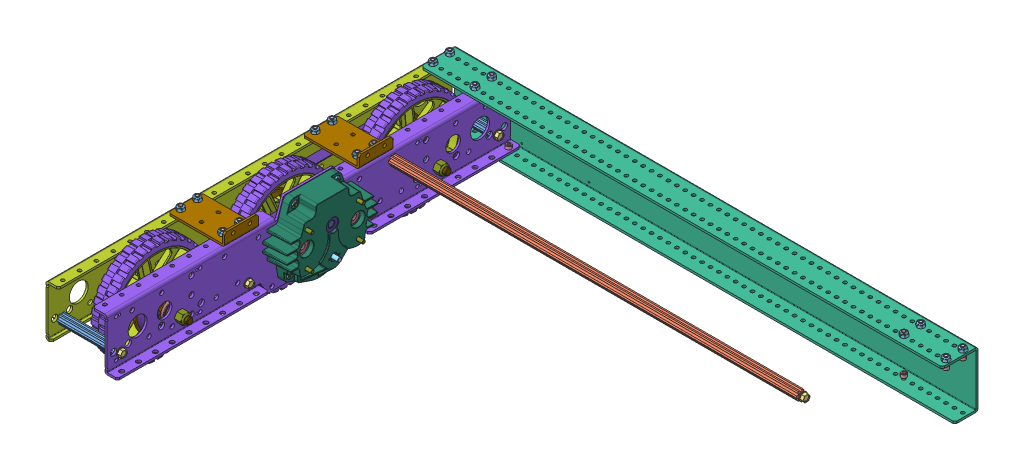
SolidWorks assembly AM14U3Wide_Half, configuration Default. Lengths in mm.
Overall size (799.92 218.82 613.54).
150 component instances, 36 part files, 25 mates.
Components (placement in the parent):
- AM14U3Wide_Frame_Half-1: AM14U3Wide_Frame_Half [Default] at (332.649 29.2384 -211.4076) size (799.34 116.33 613.54)
  - 500Churro_3.375-1: 500Churro_3.375 [Default] at (-704.85 -61.341 539.242) x (0 0 1) z (-1 0 0) size (14.66 12.7 85.72)
  - 500Churro_3.375-2: 500Churro_3.375 [Default] at (-704.85 -66.929 346.837) x (0 0 1) z (-1 0 0) size (14.66 12.7 85.72)
  - 500Churro_3.375-3: 500Churro_3.375 [Default] at (-704.85 -66.929 162.687) x (0 0 1) z (-1 0 0) size (14.66 12.7 85.72)
  - 500Churro_3.375-4: 500Churro_3.375 [Default] at (-790.575 -61.341 -29.718) x (0 0 -1) z (1 0 0) size (14.66 12.7 85.72)
  - 500Churro_24.25-1: 500Churro_24.25 [Default] at (-85.725 -15.494 127.762) x (0 0 1) z (-1 0 0) size (14.66 12.7 615.95)
  - ThreadRollingScrew_0.25-20x0.75-1: ThreadRollingScrew_0.25-20x0.75 [FHTS 0.25-20-G-0.75-C] at (-701.675 -61.341 539.242) x (-1 0 0) z (0 0.924225 0.381849) size (24.64 12.19 12.19)
  - ThreadRollingScrew_0.25-20x0.75-2: ThreadRollingScrew_0.25-20x0.75 [FHTS 0.25-20-G-0.75-C] at (-701.675 -66.929 346.837) x (-1 0 0) z (0 0.924225 0.381849) size (24.64 12.19 12.19)
  - ThreadRollingScrew_0.25-20x0.75-3: ThreadRollingScrew_0.25-20x0.75 [FHTS 0.25-20-G-0.75-C] at (-701.675 -66.929 162.687) x (-1 0 0) z (0 0.924225 0.381849) size (24.64 12.19 12.19)
  - ThreadRollingScrew_0.25-20x0.75-4: ThreadRollingScrew_0.25-20x0.75 [FHTS 0.25-20-G-0.75-C] at (-701.675 -61.341 -29.718) x (-1 0 0) z (0 0.924225 0.381849) size (24.64 12.19 12.19)
  - ThreadRollingScrew_0.25-20x0.75-5: ThreadRollingScrew_0.25-20x0.75 [FHTS 0.25-20-G-0.75-C] at (-793.75 -61.341 -29.718) size (24.64 12.19 12.19)
  - ThreadRollingScrew_0.25-20x0.75-6: ThreadRollingScrew_0.25-20x0.75 [FHTS 0.25-20-G-0.75-C] at (-793.75 -66.929 162.687) size (24.64 12.19 12.19)
  - ThreadRollingScrew_0.25-20x0.75-7: ThreadRollingScrew_0.25-20x0.75 [FHTS 0.25-20-G-0.75-C] at (-704.85 -15.494 127.762) size (24.64 12.19 12.19)
  - ThreadRollingScrew_0.25-20x0.75-8: ThreadRollingScrew_0.25-20x0.75 [FHTS 0.25-20-G-0.75-C] at (-793.75 -66.929 346.837) size (24.64 12.19 12.19)
  - ThreadRollingScrew_0.25-20x0.75-9: ThreadRollingScrew_0.25-20x0.75 [FHTS 0.25-20-G-0.75-C] at (-793.75 -61.341 539.242) size (24.64 12.19 12.19)
  - ThreadRollingScrew_0.25-20x0.75-10: ThreadRollingScrew_0.25-20x0.75 [FHTS 0.25-20-G-0.75-C] at (-82.55 -15.494 127.762) x (-1 0 0) z (0 0.116139 -0.993233) size (24.64 12.19 12.19)
  - Screw_SHCS_10-32x0.5-19: Screw_SHCS_10-32x0.5 [HX-SHCS 0.19-32x1.375x1-C] at (-781.05 -11.43 -37.338) x (0 1 0) z (0 0 1) size (17.53 7.94 7.94)
  - Screw_SHCS_10-32x0.5-20: Screw_SHCS_10-32x0.5 [HX-SHCS 0.19-32x1.375x1-C] at (-781.05 -11.43 -11.938) x (0 1 0) z (0 0 1) size (17.53 7.94 7.94)
  - Screw_SHCS_10-32x0.5-21: Screw_SHCS_10-32x0.5 [HX-SHCS 0.19-32x1.375x1-C] at (-717.55 -11.43 -37.338) x (0 1 0) z (0 0 1) size (17.53 7.94 7.94)
  - Screw_SHCS_10-32x0.5-22: Screw_SHCS_10-32x0.5 [HX-SHCS 0.19-32x1.375x1-C] at (-717.55 -11.43 -11.938) x (0 1 0) z (0 0 1) size (17.53 7.94 7.94)
  - Screw_SHCS_10-32x0.5-23: Screw_SHCS_10-32x0.5 [HX-SHCS 0.19-32x1.375x1-C] at (-781.05 -11.43 140.462) x (0 1 0) z (0 0 1) size (17.53 7.94 7.94)
  - Screw_SHCS_10-32x0.5-24: Screw_SHCS_10-32x0.5 [HX-SHCS 0.19-32x1.375x1-C] at (-781.05 -11.43 165.862) x (0 1 0) z (0 0 1) size (17.53 7.94 7.94)
  - Screw_SHCS_10-32x0.5-25: Screw_SHCS_10-32x0.5 [HX-SHCS 0.19-32x1.375x1-C] at (-717.55 -11.43 140.462) x (0 1 0) z (0 0 1) size (17.53 7.94 7.94)
  - Screw_SHCS_10-32x0.5-26: Screw_SHCS_10-32x0.5 [HX-SHCS 0.19-32x1.375x1-C] at (-717.55 -11.43 165.862) x (0 1 0) z (0 0 1) size (17.53 7.94 7.94)
  - Screw_SHCS_10-32x0.5-27: Screw_SHCS_10-32x0.5 [HX-SHCS 0.19-32x1.375x1-C] at (-781.05 -11.43 343.662) x (0 1 0) z (0 0 1) size (17.53 7.94 7.94)
  - Screw_SHCS_10-32x0.5-28: Screw_SHCS_10-32x0.5 [HX-SHCS 0.19-32x1.375x1-C] at (-781.05 -11.43 369.062) x (0 1 0) z (0 0 1) size (17.53 7.94 7.94)
  - Screw_SHCS_10-32x0.5-29: Screw_SHCS_10-32x0.5 [HX-SHCS 0.19-32x1.375x1-C] at (-717.55 -11.43 343.662) x (0 1 0) z (0 0 1) size (17.53 7.94 7.94)
  - Screw_SHCS_10-32x0.5-30: Screw_SHCS_10-32x0.5 [HX-SHCS 0.19-32x1.375x1-C] at (-717.55 -11.43 369.062) x (0 1 0) z (0 0 1) size (17.53 7.94 7.94)
  - Screw_SHCS_10-32x0.5-31: Screw_SHCS_10-32x0.5 [HX-SHCS 0.19-32x1.375x1-C] at (-692.15 -73.152 -37.338) x (0 -1 0) z (0 0 1) size (17.53 7.94 7.94)
  - Screw_SHCS_10-32x0.5-32: Screw_SHCS_10-32x0.5 [HX-SHCS 0.19-32x1.375x1-C] at (-6.35 -11.176 -11.938) x (0 1 0) z (-0.461963 0 0.886899) size (17.53 7.94 7.94)
  - Screw_SHCS_10-32x0.5-33: Screw_SHCS_10-32x0.5 [HX-SHCS 0.19-32x1.375x1-C] at (-6.35 -11.176 -37.338) x (0 1 0) z (0 0 1) size (17.53 7.94 7.94)
  - Screw_SHCS_10-32x0.5-34: Screw_SHCS_10-32x0.5 [HX-SHCS 0.19-32x1.375x1-C] at (-69.85 -11.176 -11.938) x (0 1 0) z (0 0 1) size (17.53 7.94 7.94)
  - Screw_SHCS_10-32x0.5-35: Screw_SHCS_10-32x0.5 [HX-SHCS 0.19-32x1.375x1-C] at (-69.85 -11.176 -37.338) x (0 1 0) z (0 0 1) size (17.53 7.94 7.94)
  - Screw_SHCS_10-32x0.5-36: Screw_SHCS_10-32x0.5 [HX-SHCS 0.19-32x1.375x1-C] at (-95.25 -73.406 -37.338) x (0 -1 0) z (0.251234 0 0.967926) size (17.53 7.94 7.94)
  - NylockNut_10-32-19: NylockNut_10-32 [Default] at (-717.55 0 -11.938) x (1 0 0) z (0 1 0) size (10.18 11.01 7.1)
  - NylockNut_10-32-20: NylockNut_10-32 [Default] at (-717.55 0 -37.338) x (1 0 0) z (0 1 0) size (10.18 11.01 7.1)
  - NylockNut_10-32-21: NylockNut_10-32 [Default] at (-781.05 0 -11.938) x (1 0 0) z (0 1 0) size (10.18 11.01 7.1)
  - NylockNut_10-32-22: NylockNut_10-32 [Default] at (-781.05 0 -37.338) x (1 0 0) z (0 1 0) size (10.18 11.01 7.1)
  - NylockNut_10-32-23: NylockNut_10-32 [Default] at (-781.05 -0.254 140.462) x (1 0 0) z (0 1 0) size (10.18 11.01 7.1)
  - NylockNut_10-32-24: NylockNut_10-32 [Default] at (-781.05 -0.254 165.862) x (1 0 0) z (0 1 0) size (10.18 11.01 7.1)
  - NylockNut_10-32-25: NylockNut_10-32 [Default] at (-717.55 -0.254 140.462) x (1 0 0) z (0 1 0) size (10.18 11.01 7.1)
  - NylockNut_10-32-26: NylockNut_10-32 [Default] at (-717.55 -0.254 165.862) x (1 0 0) z (0 1 0) size (10.18 11.01 7.1)
  - NylockNut_10-32-27: NylockNut_10-32 [Default] at (-781.05 -0.254 343.662) x (1 0 0) z (0 1 0) size (10.18 11.01 7.1)
  - NylockNut_10-32-28: NylockNut_10-32 [Default] at (-781.05 -0.254 369.062) x (1 0 0) z (0 1 0) size (10.18 11.01 7.1)
  - NylockNut_10-32-29: NylockNut_10-32 [Default] at (-717.55 -0.254 343.662) x (1 0 0) z (0 1 0) size (10.18 11.01 7.1)
  - NylockNut_10-32-30: NylockNut_10-32 [Default] at (-717.55 -0.254 369.062) x (1 0 0) z (0 1 0) size (10.18 11.01 7.1)
  - NylockNut_10-32-31: NylockNut_10-32 [Default] at (-692.15 -84.582 -37.338) x (1 0 0) z (0 -1 0) size (10.18 11.01 7.1)
  - NylockNut_10-32-32: NylockNut_10-32 [Default] at (-95.25 -84.582 -37.338) x (1 0 0) z (0 -1 0) size (10.18 11.01 7.1)
  - NylockNut_10-32-33: NylockNut_10-32 [Default] at (-69.85 0 -11.938) x (1 0 0) z (0 1 0) size (10.18 11.01 7.1)
  - NylockNut_10-32-34: NylockNut_10-32 [Default] at (-69.85 0 -37.338) x (1 0 0) z (0 1 0) size (10.18 11.01 7.1)
  - NylockNut_10-32-35: NylockNut_10-32 [Default] at (-6.35 0 -37.338) x (1 0 0) z (0 1 0) size (10.18 11.01 7.1)
  - NylockNut_10-32-36: NylockNut_10-32 [Default] at (-6.35 0 -11.938) x (1 0 0) z (0 1 0) size (10.18 11.01 7.1)
  - AM14U3EndPlate_Wide-1: AM14U3EndPlate_Wide [Default] at (-787.4 -81.407 -53.975) x (1 0 0) z (0 -1 0) size (787.4 53.98 84.58)
  - AM14U3OuterPlate_Wide-1: AM14U3OuterPlate_Wide [Default] at (-769.3485 -27.0221 -29.1885) x (0 0 1) z (0 -1 0) size (609.6 19.05 77.72)
  - AM14U3InnerPlate_Wide-1: AM14U3InnerPlate_Wide [Default] at (-713.7116 -19.2169 539.8409) x (0 0 -1) z (0 -1 0) size (609.6 38.1 116.33)
  - Bracket_2x3-1: Bracket_2x3 [Default] at (-787.4 -3.429 394.462) size (85.72 19.05 50.8)
  - Bracket_2x3-2: Bracket_2x3 [Default] at (-787.4 -3.429 191.262) size (85.72 19.05 50.8)
- ToughboxMini-1: ToughboxMini [Default] at (-419.5676 -40.7756 134.4552) x (0 0.001296 0.999999) z (-1 0 0) size (140.05 125.41 142.29) (flexible)
  - TBMiniSmallHexShaft-1: TBMiniSmallHexShaft [Default] at (-121.4902 80.7164 -52.3959) x (-0.931259 0.364358 0) z (0.364358 0.931259 0) size (11 38.23 9.52)
  - LargeClusterGear_Hex_50t0.375-1: LargeClusterGear_Hex_50t0.375 [Default] at (-91.0349 50.9043 -67.5597) x (-0.931259 0.364358 0) z (0 0 -1) size (65.97 66.04 10.16)
  - Bearing_FR6ZZ-1: Bearing_FR6ZZ [Default] at (-96.247 60.278 -52.5991) x (-0.893862 0.448342 0) z (0 0 1) size (24.69 24.69 7.16)
  - NylockNut_10-32-1: NylockNut_10-32 [Default] at (-129.8464 -8.0737 -56.3837) x (0.501678 0.865055 0) z (0 0 -1) size (10.18 11.01 7.1)
  - NylockNut_10-32-2: NylockNut_10-32 [Default] at (-59.2462 80.7349 -56.3837) x (0.999999 -0.001296 0) z (0 0 -1) size (10.18 11.01 7.1)
  - NylockNut_10-32-3: NylockNut_10-32 [Default] at (-122.7461 80.8172 -56.3837) x (0.500567 0.865698 0) z (0 0 -1) size (10.18 11.01 7.1)
  - NylockNut_10-32-4: NylockNut_10-32 [Default] at (-52.3764 -8.1741 -56.3837) x (-0.501678 -0.865055 0) z (0 0 -1) size (10.18 11.01 7.1)
  - Washer_5-16-1: Washer_5-16 [Default] at (-52.3162 38.3079 -77.7705) x (-0.418041 0.908428 0) z (0 0 -1) size (17.53 17.53 1.47)
  - Washer_5-16-2: Washer_5-16 [Default] at (-52.3162 38.3079 -76.2973) x (0.897267 -0.441488 0) z (0 0 -1) size (17.53 17.53 1.47)
  - Washer_5-16-3: Washer_5-16 [Default] at (-129.7861 38.4083 -77.7705) x (-0.990116 0.140253 0) z (0 0 1) size (17.53 17.53 1.47)
  - Washer_5-16-4: Washer_5-16 [Default] at (-129.7861 38.4083 -79.2437) x (-0.681761 0.731575 0) z (0 0 1) size (17.53 17.53 1.47)
  - CIMGear_14t8mm-1: CIMGear_14t8mm [Default] at (-52.3162 38.3079 -63.5973) x (0.843315 0.537419 0) z (0 0 -1) size (20.03 20.32 12.7)
  - CIMGear_14t8mm-2: CIMGear_14t8mm [Default] at (-129.7861 38.4083 -63.5973) x (0.986729 -0.162375 0) z (0 0 -1) size (20.03 20.32 12.7)
  - TBMiniHousing-1: TBMiniHousing [Default] at (-91.0876 10.1882 -86.3557) x (0.999999 -0.001296 0) z (0 0 1) size (139.9 118.55 41.54)
  - Screw_SHCS_10-32x0.625-1: Screw_SHCS_10-32x0.625 [Default] at (-52.2832 63.7078 -74.4685) x (-0.564778 -0.825243 0) z (-0.825243 0.564778 0) size (7.82 20.65 7.82)
  - Screw_SHCS_10-32x0.625-2: Screw_SHCS_10-32x0.625 [Default] at (-122.7461 80.8172 -42.5915) x (0.507484 -0.861661 0) z (-0.861661 -0.507484 0) size (7.82 20.65 7.82)
  - Screw_SHCS_10-32x0.625-3: Screw_SHCS_10-32x0.625 [Default] at (-52.3764 -8.1741 -42.5915) x (0.507484 -0.861661 0) z (-0.861661 -0.507484 0) size (7.82 20.65 7.82)
  - Screw_SHCS_10-32x0.625-4: Screw_SHCS_10-32x0.625 [Default] at (-129.8464 -8.0737 -42.5915) x (0.507484 -0.861661 0) z (-0.861661 -0.507484 0) size (7.82 20.65 7.82)
  - Screw_SHCS_10-32x0.625-5: Screw_SHCS_10-32x0.625 [Default] at (-59.2462 80.7349 -42.5915) x (0.740711 -0.671824 0) z (-0.671824 -0.740711 0) size (7.82 20.65 7.82)
  - Screw_SHCS_10-32x0.625-6: Screw_SHCS_10-32x0.625 [Default] at (-52.3491 12.9079 -74.4685) x (-0.564778 -0.825243 0) z (-0.825243 0.564778 0) size (7.82 20.65 7.82)
  - Screw_SHCS_10-32x0.625-7: Screw_SHCS_10-32x0.625 [Default] at (-129.7532 63.8083 -74.4685) x (-0.966277 -0.257503 0) z (-0.257503 0.966277 0) size (7.82 20.65 7.82)
  - Screw_SHCS_10-32x0.625-8: Screw_SHCS_10-32x0.625 [Default] at (-129.819 13.0083 -74.4685) x (-0.99652 0.083357 0) z (0.083357 0.99652 0) size (7.82 20.65 7.82)
  - Bearing_R6ZZ-3: Bearing_R6ZZ [Default] at (-91.0349 50.9043 -84.8317) x (0.958138 -0.286306 0) z (0 0 1) size (22.23 22.23 7.11)
  - Bearing_R6ZZ-4: Bearing_R6ZZ [Default] at (-91.0876 10.1882 -84.8317) x (-0.661529 0.74992 0) z (0 0 1) size (22.23 22.23 7.11)
  - RetainingClip-1: RetainingClip [Default] at (-129.7861 38.4083 -63.5973) x (0 0 1) z (-1 0 0) size (1.09 14.83 14.83)
  - RetainingClip-2: RetainingClip [Default] at (-52.3162 38.3079 -63.5973) x (0 0 1) z (-1 0 0) size (1.09 14.83 14.83)
  - ExternalKlipring-1: ExternalKlipring [Default] at (-91.0876 10.1882 -64.4355) x (0.996411 -0.084651 0) z (0 0 1) size (19.07 20.96 1.27)
  - HexBearing_FR8ZZ-1: HexBearing_FR8ZZ [Default] at (-91.0876 10.1882 -44.6717) x (0.58483 -0.811156 0) z (0 0 -1) size (31.12 31.12 7.93)
  - SmallClusterGear_Hex_16t0.375-1: SmallClusterGear_Hex_16t0.375 [Default] at (-91.0349 50.9043 -67.5597) x (0 0 1) z (-0.781173 -0.624315 0) size (15.19 22.57 22.57)
  - LargeOutputGear_Hex_48t0.5-1: LargeOutputGear_Hex_48t0.5 [Default] at (-91.0876 10.1882 -63.1655) x (0 0 1) z (0.410066 0.912056 0) size (10.21 63.42 63.42)
  - TBMiniHexOutputShaft-2: TBMiniHexOutputShaft [Default] at (-82.2056 -30.6334 -52.3197) x (0.58483 -0.811156 0) z (-0.811156 -0.58483 0) size (14.66 142.29 12.7)
- Bearing_Hex_FR8ZZ-1: Bearing_Hex_FR8ZZ [Default] at (-464.3293 -30.7056 43.3544) x (0 -0.10219 -0.994765) z (1 0 0) size (31.12 31.12 7.93)
- Wheel_6inHiGrip_Center-1: Wheel_6inHiGrip_Center [Default] at (-383.2007 58.6676 167.6224) x (-1 0 0) z (0 -0.912587 -0.408883) size (81.42 191.55 191.55)
  - Wheel_6inHiGrip-1: Wheel_6inHiGrip [Default] at (83.7987 67.439 110.9939) size (35.05 191.55 191.55)
    - Wheel_6inHiGrip_Wheel-1: Wheel_6inHiGrip_Wheel [Default] at (-52.6446 9.4231 21.378) size (35.05 132.08 132.08)
    - Wheel_6inHiGrip_Tread-1: Wheel_6inHiGrip_Tread [Default] at (-65.3446 9.4231 21.378) x (0 -0.304368 -0.952555) z (1 0 0) size (152.4 152.4 25.58)
  - HalfPulley_42t5mm-1: HalfPulley_42t5mm [Default] at (47.6006 76.862 132.3719) x (1 0 0) z (0 -0.5 0.866025) size (13 74.23 74.23)
  - HalfPulley_42t5mm-2: HalfPulley_42t5mm [Default] at (64.263 76.862 132.3719) x (-1 0 0) z (0 -0.499927 0.866067) size (13 74.23 74.23)
  - ThreadFormingScrew_10-24x1.25-1: ThreadFormingScrew_10-24x1.25 [93882A213] at (63.247 76.8605 108.5602) x (0 0 -1) z (1 0 0) size (10.52 10.52 35.59)
  - ThreadFormingScrew_10-24x1.25-2: ThreadFormingScrew_10-24x1.25 [93882A213] at (63.247 97.4833 120.4656) x (0 0 -1) z (1 0 0) size (10.52 10.52 35.59)
  - ThreadFormingScrew_10-24x1.25-3: ThreadFormingScrew_10-24x1.25 [93882A213] at (63.247 56.2398 144.2799) x (0 0 -1) z (1 0 0) size (10.52 10.52 35.59)
  - ThreadFormingScrew_10-24x1.25-4: ThreadFormingScrew_10-24x1.25 [93882A213] at (63.247 76.8625 156.1852) x (0 -0.95788 -0.287168) z (1 0 0) size (10.52 10.52 35.59)
  - ThreadFormingScrew_10-24x1.25-5: ThreadFormingScrew_10-24x1.25 [93882A213] at (63.247 97.4843 144.2781) x (0 -0.868976 0.494854) z (1 0 0) size (10.52 10.52 35.59)
  - ThreadFormingScrew_10-24x1.25-6: ThreadFormingScrew_10-24x1.25 [93882A213] at (63.247 56.2388 120.4674) x (0 -0.748729 -0.662876) z (1 0 0) size (10.52 10.52 35.59)
  - HalfPulley_42t5mm-3: HalfPulley_42t5mm [Default] at (-1.9548 76.8628 132.3714) x (1 0 0) z (0 -1 -0.000063) size (13 74.23 74.23)
  - HalfPulley_42t5mm-4: HalfPulley_42t5mm [Default] at (14.7076 76.8628 132.3714) x (-1 0 0) z (0 -1 0.000021) size (13 74.23 74.23)
  - HexHub_500EX-1: HexHub_500EX [Default] at (-8.3048 76.8628 132.3714) x (0 -0.866025 -0.5) z (0 -0.5 0.866025) size (55.37 25.4 51.33)
  - ThreadFormingScrew_10-24x1.25-7: ThreadFormingScrew_10-24x1.25 [93882A213] at (-5.2568 97.485 120.4652) x (0 0 1) z (-1 0 0) size (10.52 10.52 35.59)
  - ThreadFormingScrew_10-24x1.25-8: ThreadFormingScrew_10-24x1.25 [93882A213] at (-5.2568 76.8628 108.5589) x (0 0 1) z (-1 0 0) size (10.52 10.52 35.59)
  - ThreadFormingScrew_10-24x1.25-9: ThreadFormingScrew_10-24x1.25 [93882A213] at (-5.2568 56.2406 120.4652) x (0 0 1) z (-1 0 0) size (10.52 10.52 35.59)
  - ThreadFormingScrew_10-24x1.25-10: ThreadFormingScrew_10-24x1.25 [93882A213] at (-5.2568 97.485 144.2777) x (0 -0.99374 -0.111715) z (-1 0 0) size (10.52 10.52 35.59)
  - ThreadFormingScrew_10-24x1.25-11: ThreadFormingScrew_10-24x1.25 [93882A213] at (-5.2568 56.2406 144.2777) x (0 -0.138911 0.990305) z (-1 0 0) size (10.52 10.52 35.59)
  - ThreadFormingScrew_10-24x1.25-12: ThreadFormingScrew_10-24x1.25 [93882A213] at (-5.2568 76.8628 156.1839) x (0 -0.98811 -0.15375) z (-1 0 0) size (10.52 10.52 35.59)
  - Spacer_Hex_0.57x0.5-1: Spacer_Hex_0.57x0.5 [Default] at (57.8495 76.862 132.3719) x (0 -0.866025 -0.5) z (0 -0.5 0.866025) size (28.55 14.48 28.55)
- Wheel-6inHiGrip_Outer-1: Wheel-6inHiGrip_Outer [Default] at (-446.6875 116.3359 190.1372) x (1 0 0) z (0 -0.97899 -0.203906) size (85.56 191.55 191.55)
  - Wheel_6inHiGrip-1: Wheel_6inHiGrip [Default] at (83.7987 67.439 110.9939) size (35.05 191.55 191.55)
    - Wheel_6inHiGrip_Wheel-1: Wheel_6inHiGrip_Wheel [Default] at (-52.6446 9.4231 21.378) size (35.05 132.08 132.08)
    - Wheel_6inHiGrip_Tread-1: Wheel_6inHiGrip_Tread [Default] at (-65.3446 9.4231 21.378) x (0 -0.304368 -0.952555) z (1 0 0) size (152.4 152.4 25.58)
  - HalfPulley_42t5mm-1: HalfPulley_42t5mm [Default] at (47.6006 76.862 132.3719) x (1 0 0) z (0 -0.5 0.866025) size (13 74.23 74.23)
  - HalfPulley_42t5mm-2: HalfPulley_42t5mm [Default] at (64.263 76.862 132.3719) x (-1 0 0) z (0 -0.499927 0.866067) size (13 74.23 74.23)
  - Bearing_1614ZZ-1: Bearing_1614ZZ [Default] at (62.612 76.862 132.3719) x (0 -0.157148 -0.987575) z (-1 0 0) size (28.57 28.57 9.53)
  - Bearing_1614ZZ-2: Bearing_1614ZZ [Default] at (15.2791 76.862 132.3719) x (0 0 -1) z (1 0 0) size (28.57 28.57 9.53)
  - ThreadFormingScrew_10-24x1.25-1: ThreadFormingScrew_10-24x1.25 [93882A213] at (63.247 76.8605 108.5602) x (0 0 -1) z (1 0 0) size (10.52 10.52 35.59)
  - ThreadFormingScrew_10-24x1.25-2: ThreadFormingScrew_10-24x1.25 [93882A213] at (63.247 97.4833 120.4656) x (0 0 -1) z (1 0 0) size (10.52 10.52 35.59)
  - ThreadFormingScrew_10-24x1.25-3: ThreadFormingScrew_10-24x1.25 [93882A213] at (63.247 56.2398 144.2799) x (0 0 -1) z (1 0 0) size (10.52 10.52 35.59)
  - ThreadFormingScrew_10-24x1.25-4: ThreadFormingScrew_10-24x1.25 [93882A213] at (63.247 76.8625 156.1852) x (0 -0.95788 -0.287168) z (1 0 0) size (10.52 10.52 35.59)
  - ThreadFormingScrew_10-24x1.25-5: ThreadFormingScrew_10-24x1.25 [93882A213] at (63.247 97.4843 144.2781) x (0 -0.868976 0.494854) z (1 0 0) size (10.52 10.52 35.59)
  - ThreadFormingScrew_10-24x1.25-6: ThreadFormingScrew_10-24x1.25 [93882A213] at (63.247 56.2388 120.4674) x (0 -0.977348 -0.211637) z (1 0 0) size (10.52 10.52 35.59)
  - Spacer_0.28x0.382-1: Spacer_0.28x0.382 [Default] at (74.4865 76.862 132.3719) x (0 -0.35357 0.935408) z (-1 0 0) size (13.16 13.16 7.11)
  - Spacer_0.85x0.38-1: Spacer_0.85x0.38 [Default] at (-11.0734 76.862 132.3719) x (0 0 -1) z (1 0 0) size (19.05 19.05 21.59)
- Wheel-6inHiGrip_Outer-2: Wheel-6inHiGrip_Outer [Default] at (-383.2744 96.4564 -63.8834) x (-1 0 0) z (0 -0.996405 -0.084723) size (85.56 191.55 191.55)
  - Wheel_6inHiGrip-1: Wheel_6inHiGrip [Default] at (83.7987 67.439 110.9939) size (35.05 191.55 191.55)
    - Wheel_6inHiGrip_Wheel-1: Wheel_6inHiGrip_Wheel [Default] at (-52.6446 9.4231 21.378) size (35.05 132.08 132.08)
    - Wheel_6inHiGrip_Tread-1: Wheel_6inHiGrip_Tread [Default] at (-65.3446 9.4231 21.378) x (0 -0.304368 -0.952555) z (1 0 0) size (152.4 152.4 25.58)
  - HalfPulley_42t5mm-1: HalfPulley_42t5mm [Default] at (47.6006 76.862 132.3719) x (1 0 0) z (0 -0.5 0.866025) size (13 74.23 74.23)
  - HalfPulley_42t5mm-2: HalfPulley_42t5mm [Default] at (64.263 76.862 132.3719) x (-1 0 0) z (0 -0.499927 0.866067) size (13 74.23 74.23)
  - Bearing_1614ZZ-1: Bearing_1614ZZ [Default] at (62.612 76.862 132.3719) x (0 -0.157148 -0.987575) z (-1 0 0) size (28.57 28.57 9.53)
  - Bearing_1614ZZ-2: Bearing_1614ZZ [Default] at (15.2791 76.862 132.3719) x (0 0 -1) z (1 0 0) size (28.57 28.57 9.53)
  - ThreadFormingScrew_10-24x1.25-1: ThreadFormingScrew_10-24x1.25 [93882A213] at (63.247 76.8605 108.5602) x (0 0 -1) z (1 0 0) size (10.52 10.52 35.59)
  - ThreadFormingScrew_10-24x1.25-2: ThreadFormingScrew_10-24x1.25 [93882A213] at (63.247 97.4833 120.4656) x (0 0 -1) z (1 0 0) size (10.52 10.52 35.59)
  - ThreadFormingScrew_10-24x1.25-3: ThreadFormingScrew_10-24x1.25 [93882A213] at (63.247 56.2398 144.2799) x (0 0 -1) z (1 0 0) size (10.52 10.52 35.59)
  - ThreadFormingScrew_10-24x1.25-4: ThreadFormingScrew_10-24x1.25 [93882A213] at (63.247 76.8625 156.1852) x (0 -0.95788 -0.287168) z (1 0 0) size (10.52 10.52 35.59)
  - ThreadFormingScrew_10-24x1.25-5: ThreadFormingScrew_10-24x1.25 [93882A213] at (63.247 97.4843 144.2781) x (0 -0.868976 0.494854) z (1 0 0) size (10.52 10.52 35.59)
  - ThreadFormingScrew_10-24x1.25-6: ThreadFormingScrew_10-24x1.25 [93882A213] at (63.247 56.2388 120.4674) x (0 -0.977348 -0.211637) z (1 0 0) size (10.52 10.52 35.59)
  - Spacer_0.28x0.382-1: Spacer_0.28x0.382 [Default] at (74.4865 76.862 132.3719) x (0 -0.35357 0.935408) z (-1 0 0) size (13.16 13.16 7.11)
  - Spacer_0.85x0.38-1: Spacer_0.85x0.38 [Default] at (-11.0734 76.862 132.3719) x (0 0 -1) z (1 0 0) size (19.05 19.05 21.59)
- NylockNut_0.375-16-1: NylockNut_0.375-16 [91831A127] at (-369.026 -28.9276 238.3929) x (0 -1 0) z (0 0 1) size (14.29 12 16.5)
- NylockNut_0.375-16-2: NylockNut_0.375-16 [91831A127] at (-369.026 -28.9276 -151.6841) x (0 -1 0) z (0 0 1) size (14.29 12 16.5)
- Belt_15mm131t_Wide-1: Belt_15mm131t_Wide [Default] at (-384.0869 -30.7056 43.3544) x (0 0.009116 0.999958) z (-1 0 0) size (264.24 69.19 15)
- Belt_15mm131t_Wide-2: Belt_15mm131t_Wide [Default] at (-445.875 -30.7056 43.3544) x (0 0.009116 -0.999958) z (1 0 0) size (264.24 69.19 15)
- HHSBolt_0.375-16x4.25-1: HHSBolt_0.375-16x4.25 [HFBOLT 0.375-16x2.5x1-C] at (-467.2732 -28.9276 238.3929) x (1 0 0) z (0 -0.996292 -0.086036) size (114.12 16.48 14.27)
- HHSBolt_0.375-16x4.25-2: HHSBolt_0.375-16x4.25 [HFBOLT 0.375-16x2.5x1-C] at (-467.2732 -28.9276 -151.6841) size (114.12 16.48 14.27)
Mates (geometry in assembly coordinates):
- Concentric1: concentric anti-aligned: cylinder of AM14U3Wide_Frame_Half-1/AM14U3InnerPlate_Wide-1 through (-372.201 -30.7056 43.3544) axis (1 0 0) radius 14.2875; cylinder of ToughboxMini-1/HexBearing_FR8ZZ-1 through (-366.9686 -30.7056 43.3544) axis (-1 0 0) radius 14.2875
- Parallel1: parallel: plane of AM14U3Wide_Frame_Half-1/AM14U3InnerPlate_Wide-1 through (-369.026 49.3044 -4.2706) normal (0 1 0); line of ToughboxMini-1/TBMiniHousing-1 through (-368.5002 48.8617 11.6044) axis (0 0 1)
- Coincident2: coincident anti-aligned: plane of AM14U3Wide_Frame_Half-1/AM14U3InnerPlate_Wide-1 through (-369.026 21.8724 449.7544) normal (1 0 0); plane of ToughboxMini-1/TBMiniHousing-1 through (-369.026 -30.7056 43.3544) normal (-1 0 0)
- Concentric21: concentric aligned: cylinder of AM14U3Wide_Frame_Half-1/AM14U3OuterPlate_Wide-1 through (-457.926 -30.7056 43.3544) axis (-1 0 0) radius 14.2875; cylinder of Bearing_Hex_FR8ZZ-1 through (-456.402 -30.7056 43.3544) axis (-1 0 0) radius 13.97
- Coincident31: coincident anti-aligned: plane of AM14U3Wide_Frame_Half-1/AM14U3OuterPlate_Wide-1 through (-457.926 21.8724 -363.0456) normal (1 0 0); plane of Bearing_Hex_FR8ZZ-1 through (-457.926 -32.1332 29.4576) normal (-1 0 0)
- Coincident4: coincident anti-aligned: plane of ToughboxMini-1/TBMiniHexOutputShaft-2 through (-341.848 -24.7635 39.0585) normal (0 0.408883 -0.912587); plane of Bearing_Hex_FR8ZZ-1 through (-456.402 -24.7635 39.0585) normal (0 -0.408883 0.912587)
- Concentric3: concentric anti-aligned: cylinder of ToughboxMini-1/HexBearing_FR8ZZ-1 through (-366.9686 -30.7056 43.3544) axis (-1 0 0) radius 14.2875; cylinder of Wheel_6inHiGrip_Center-1/Spacer_Hex_0.57x0.5-1 through (-455.5282 -30.7056 43.3544) axis (1 0 0) radius 14.2748
- Parallel2: parallel anti-aligned: plane of ToughboxMini-1/TBMiniHexOutputShaft-2 through (-341.848 -24.7635 39.0585) normal (0 0.408883 -0.912587); plane of Wheel_6inHiGrip_Center-1/HexHub_500EX-1 through (-374.8959 -24.7509 39.0494) normal (0 -0.408883 0.912587)
- Coincident6: coincident anti-aligned: plane of ToughboxMini-1/HexBearing_FR8ZZ-1 through (-374.8959 -30.7056 43.3544) normal (-1 0 0); plane of Wheel_6inHiGrip_Center-1/HexHub_500EX-1 through (-374.8959 -30.7049 43.3539) normal (1 0 0)
- Concentric4: concentric aligned: cylinder of AM14U3Wide_Frame_Half-1/AM14U3InnerPlate_Wide-1 through (-391.251 -28.9276 238.3929) axis (1 0 0) radius 4.826; cylinder of Wheel-6inHiGrip_Outer-1/Spacer_0.28x0.382-1 through (-379.313 -28.9276 238.3929) axis (1 0 0) radius 6.5786
- Coincident7: coincident anti-aligned: plane of AM14U3Wide_Frame_Half-1/AM14U3InnerPlate_Wide-1 through (-372.201 21.8724 449.7544) normal (-1 0 0); plane of Wheel-6inHiGrip_Outer-1/Spacer_0.28x0.382-1 through (-372.201 -28.9276 238.3929) normal (1 0 0)
- Concentric5: concentric anti-aligned: cylinder of AM14U3Wide_Frame_Half-1/AM14U3InnerPlate_Wide-1 through (-391.251 -28.9276 -151.6841) axis (1 0 0) radius 4.826; cylinder of Wheel-6inHiGrip_Outer-2/Spacer_0.28x0.382-1 through (-450.6489 -28.9276 -151.6841) axis (-1 0 0) radius 6.5786
- Coincident8: coincident anti-aligned: plane of AM14U3Wide_Frame_Half-1/AM14U3InnerPlate_Wide-1 through (-372.201 21.8724 449.7544) normal (-1 0 0); plane of Wheel-6inHiGrip_Outer-2/Spacer_0.85x0.38-1 through (-372.201 -28.9276 -151.6841) normal (1 0 0)
- Coincident11: coincident anti-aligned: plane of AM14U3Wide_Frame_Half-1/AM14U3InnerPlate_Wide-1 through (-369.026 21.8724 449.7544) normal (1 0 0); plane of NylockNut_0.375-16-2 through (-369.026 -21.7838 -164.0574) normal (-1 0 0)
- Coincident12: coincident anti-aligned: plane of AM14U3Wide_Frame_Half-1/AM14U3InnerPlate_Wide-1 through (-369.026 21.8724 449.7544) normal (1 0 0); plane of NylockNut_0.375-16-1 through (-369.026 -21.7838 226.0196) normal (-1 0 0)
- Concentric10: concentric anti-aligned: cylinder of Wheel-6inHiGrip_Outer-1/Spacer_0.85x0.38-1 through (-436.1709 -28.9276 238.3929) axis (-1 0 0) radius 9.525; cylinder of Belt_15mm131t_Wide-1 through (-399.0869 -28.9276 238.3929) axis (1 0 0) radius 33.4264
- Concentric11: concentric anti-aligned: cylinder of Bearing_Hex_FR8ZZ-1 through (-456.402 -30.7056 43.3544) axis (-1 0 0) radius 14.2875; cylinder of Belt_15mm131t_Wide-1 through (-399.0869 -30.7056 43.3544) axis (1 0 0) radius 33.4264
- Coincident13: coincident anti-aligned: plane of Wheel-6inHiGrip_Outer-1/HalfPulley_42t5mm-1 through (-399.0869 -28.9276 238.3929) normal (1 0 0); plane of Belt_15mm131t_Wide-1 through (-399.0869 -30.7056 43.3544) normal (-1 0 0)
- Concentric12: concentric anti-aligned: cylinder of Wheel-6inHiGrip_Outer-2/Spacer_0.85x0.38-1 through (-393.791 -28.9276 -151.6841) axis (1 0 0) radius 9.525; cylinder of Belt_15mm131t_Wide-2 through (-430.875 -28.9276 -151.6841) axis (-1 0 0) radius 33.4264
- Concentric13: concentric anti-aligned: circle of Bearing_Hex_FR8ZZ-1; cylinder of Belt_15mm131t_Wide-2 through (-430.875 -30.7056 43.3544) axis (-1 0 0) radius 33.4264
- Coincident14: coincident anti-aligned: plane of Wheel-6inHiGrip_Outer-2/HalfPulley_42t5mm-1 through (-430.875 -28.9276 -151.6841) normal (-1 0 0); plane of Belt_15mm131t_Wide-2 through (-430.875 -30.7056 43.3544) normal (1 0 0)
- Concentric72: concentric aligned: cylinder of AM14U3Wide_Frame_Half-1/AM14U3OuterPlate_Wide-1 through (-349.975 -28.9276 238.3929) axis (-1 0 0) radius 4.826; cylinder of HHSBolt_0.375-16x4.25-1 through (-467.2732 -28.9276 238.3929) axis (-1 0 0) radius 4.7625
- Coincident102: coincident anti-aligned: plane of AM14U3Wide_Frame_Half-1/AM14U3OuterPlate_Wide-1 through (-461.101 21.8724 -363.0456) normal (-1 0 0); plane of HHSBolt_0.375-16x4.25-1 through (-461.101 -29.6366 246.6039) normal (1 0 0)
- Concentric731: concentric aligned: cylinder of AM14U3Wide_Frame_Half-1/AM14U3OuterPlate_Wide-1 through (-349.975 -28.9276 -151.6841) axis (-1 0 0) radius 4.826; cylinder of HHSBolt_0.375-16x4.25-2 through (-467.2732 -28.9276 -151.6841) axis (-1 0 0) radius 7.1374
- Coincident1031: coincident anti-aligned: plane of AM14U3Wide_Frame_Half-1/AM14U3OuterPlate_Wide-1 through (-461.101 21.8724 -363.0456) normal (-1 0 0); plane of HHSBolt_0.375-16x4.25-2 through (-461.101 -20.686 -151.6841) normal (1 0 0)
